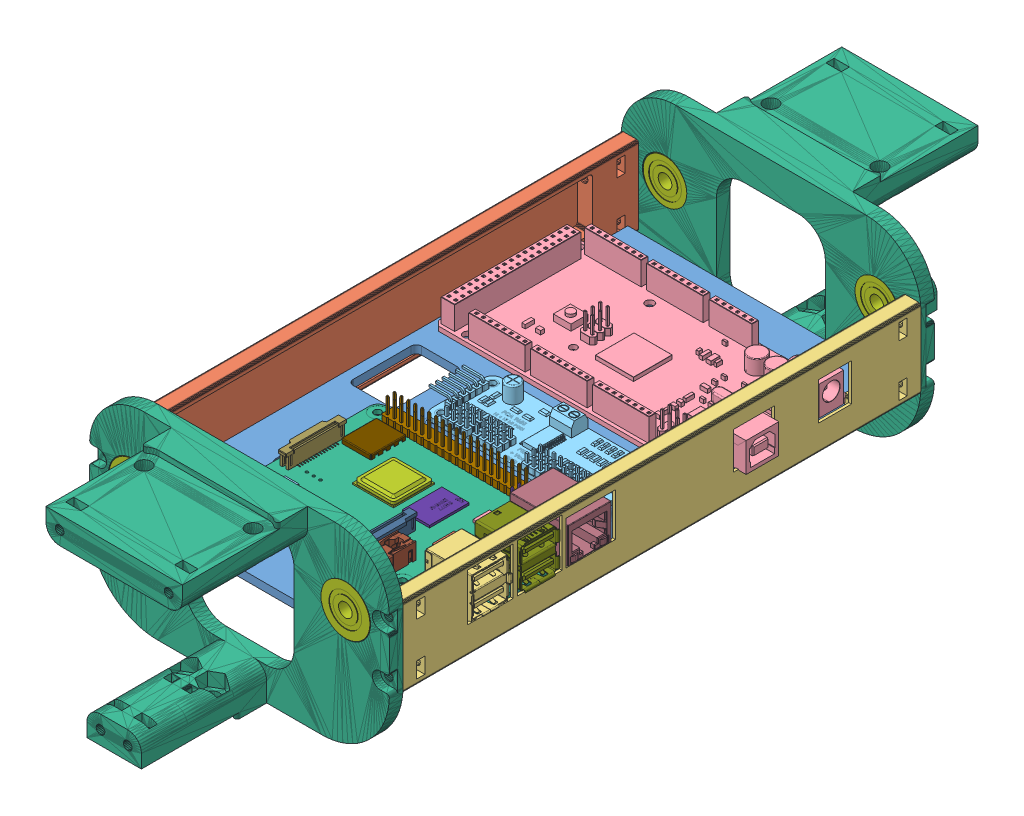
SolidWorks assembly Chase Assembly, configuration Default. Lengths in mm.
Overall size (112.8 70 292).
68 component instances, 28 part files, 131 mates.
Components (placement in the parent):
- 1_2MCU_Plate-1: 1_2MCU_Plate [Default] at (22.3647 94.0168 229.1495) size (106 5.81 180)
- 2_2MCU_Left_side_plate-1: 2_2MCU_Left_side_plate [Default] at (18.1147 57.0168 99.1495) x (1 0 0) z (0 -1 0) size (6.5 190 29)
- 3_2MCU_Right_side_plate-1: 3_2MCU_Right_side_plate [Default] at (121.6147 57.0168 169.1495) x (-1 0 0) z (0 -1 0) size (6.5 190 29)
- ArduinoMega-1: ArduinoMega [Default] at (70.5126 101.4678 88.5891) x (1 0 0) z (0 -1 0) size (107.95 53.42 12.95)
- _Hex_Screws-1: _Hex_Screws [H M3x8] at (55.5647 101.4678 97.3157) x (-0.837169 0 -0.546944) z (-0.546944 0 0.837169) size (5.5 10 6.35) (hidden)
- _Hex_Screws-2: _Hex_Screws [H M3x8] at (55.5647 101.4678 69.2995) x (0.837169 0 0.546944) z (0.546944 0 -0.837169) size (5.5 10 6.35) (hidden)
- 4_M3_nut-1: 4_M3_nut [Default] at (55.5655 95.0168 69.2614) x (0.855198 0 0.518302) z (-0.518302 0 0.855198) size (6 2.34 5.2) (hidden)
- 4_M3_nut-2: 4_M3_nut [Default] at (55.5332 95.0168 97.2415) x (-0.878773 0 0.47724) z (-0.47724 0 -0.878773) size (6 2.34 5.2) (hidden)
- 12Channel PWM-1: 12Channel PWM [Default] at (79.9147 99.8168 132.7995) x (0 0 -1) z (1 0 0) size (25.4 7.55 66.7)
- _M2_nut-1: _M2_nut [Default] at (51.9456 95.5168 142.2881) x (-0.74075 0 -0.671781) z (0 -1 0) size (4.67 4.62 1.63) (hidden)
- _M2_nut-2: _M2_nut [Default] at (107.8452 93.9168 142.288) x (-0.738205 0 -0.674577) z (0 1 0) size (4.67 4.62 1.63) (hidden)
- _M2_nut-3: _M2_nut [Default] at (107.8453 93.9168 123.488) x (-0.739008 0 -0.673697) z (0 1 0) size (4.67 4.62 1.63) (hidden)
- _M2_nut-4: _M2_nut [Default] at (51.8785 93.9168 123.4273) x (-0.741456 0 -0.671001) z (0 1 0) size (4.67 4.62 1.63) (hidden)
- _Hex_Screws-3: _Hex_Screws [H M2x8] at (51.9647 101.3268 142.1995) x (0.837169 0 0.546944) z (0.546944 0 -0.837169) size (4 9.4 4.62) (hidden)
- _Hex_Screws-4: _Hex_Screws [H M2x8] at (107.8647 101.3268 123.3995) x (0.837169 0 0.546944) z (0.546944 0 -0.837169) size (4 9.4 4.62) (hidden)
- _Hex_Screws-5: _Hex_Screws [H M2x8] at (51.9647 101.3268 123.3995) x (0.837169 0 0.546944) z (0.546944 0 -0.837169) size (4 9.4 4.62) (hidden)
- _Hex_Screws-6: _Hex_Screws [H M2x8] at (107.8647 101.3268 142.1995) x (0.837169 0 0.546944) z (0.546944 0 -0.837169) size (4 9.4 4.62) (hidden)
- _Hex_Screws-11: _Hex_Screws [H M2x8] at (40.2647 101.4168 153.7995) x (0.837169 0 0.546944) z (0.546944 0 -0.837169) size (4 9.4 4.62) (hidden)
- _Hex_Screws-12: _Hex_Screws [H M2x8] at (98.2647 101.4068 153.7995) x (0.837169 0 0.546944) z (0.546944 0 -0.837169) size (4 9.4 4.62) (hidden)
- _Hex_Screws-13: _Hex_Screws [H M2x8] at (40.2647 101.4068 202.7995) x (0.837169 0 0.546944) z (0.546944 0 -0.837169) size (4 9.4 4.62) (hidden)
- _Hex_Screws-14: _Hex_Screws [H M2x8] at (98.2647 101.4168 202.7995) x (0.837169 0 0.546944) z (0.546944 0 -0.837169) size (4 9.4 4.62) (hidden)
- _M2_nut-9: _M2_nut [Default] at (98.2838 93.9168 153.7109) x (-0.741324 0 -0.671147) z (0 1 0) size (4.67 4.62 1.63) (hidden)
- _M2_nut-10: _M2_nut [Default] at (40.2838 93.9168 202.711) x (-0.74083 0 -0.671693) z (0 1 0) size (4.67 4.62 1.63) (hidden)
- _M2_nut-11: _M2_nut [Default] at (98.2457 93.9168 202.8881) x (-0.741502 0 -0.670951) z (0 1 0) size (4.67 4.62 1.63) (hidden)
- _M2_nut-12: _M2_nut [Default] at (40.3319 95.5168 153.8603) x (-0.741456 0 -0.671001) z (0 -1 0) size (4.67 4.62 1.63) (hidden)
- Raspberry Pi 4 Model B-1: Raspberry Pi 4 Model B [Default] at (79.2647 100.6168 178.2995) size (89 19.92 58.4)
  - Raspberry Pi 4 Model B.STEP-1: Raspberry Pi 4 Model B.STEP [Default] at origin size (89 19.92 58.4)
    - PCB, RPi4ModelB.STEP-1: PCB, RPi4ModelB.STEP [Default] at origin size (85 1.6 56)
    - Broadcom BCM2711B0 CPU, RPi4ModelB.STEP-1: Broadcom BCM2711B0 CPU, RPi4ModelB.STEP [Default] at (-13.25 0.8 -4.5) size (15 2.3 15)
    - 2.54 mm DUPONT MALE PIN HEADER, POE, 2X2, RPi4ModelB.STEP-1: 2.54 mm DUPONT MALE PIN HEADER, POE, 2X2, RPi4ModelB.STEP [Default] at (19 0.8 -18.36) size (5.08 11.3 5.08)
    - 2.54 mm DUPONT MALE PIN HEADER, IO, 2X20, RPi4ModelB.STEP-1: 2.54 mm DUPONT MALE PIN HEADER, IO, 2X20, RPi4ModelB.STEP [Default] at (-10 0.8 -24.5) size (50.8 11.3 5.08)
    - Camera Connector, RPi4ModelB.STEP-1: Camera Connector, RPi4ModelB.STEP [Default] at (4 0.8 16.5) x (0 0 -1) z (1 0 0) size (22.4 5.68 5.07)
    - Microphone Plug, RPi4ModelB.STEP-1: Microphone Plug, RPi4ModelB.STEP [Default] at (11.5 0.8 21.65) size (7.23 7.55 15)
    - Display Connector, RPi4ModelB.STEP-1: Display Connector, RPi4ModelB.STEP [Default] at (-38.5 0.8 0) x (0 0 1) z (-1 0 0) size (22.4 5.68 5.07)
    - Gigabit Ethernet Port, RPi4ModelB.STEP-1: Gigabit Ethernet Port, RPi4ModelB.STEP [Default] at (45.5 7.55 -17.75) x (0 0 -1) z (1 0 0) size (16.33 17.24 21.6)
    - Female Micro HDMI Connector, RPi4ModelB.STEP-1: Female Micro HDMI Connector, RPi4ModelB.STEP [Default] at (-3 0.8 27.3875) size (6.5 3.51 7.5)
    - Female Micro HDMI Connector, RPi4ModelB.STEP-2: Female Micro HDMI Connector, RPi4ModelB.STEP [Default] at (-16.5 0.8 27.3875) size (6.5 3.51 7.5)
    - Female USB Type C Connector, RPi4ModelB.STEP-1: Female USB Type C Connector, RPi4ModelB.STEP [Default] at (-31.3 0.8 26.5419) size (8.94 3.96 7.9)
    - 2X USB3.0 PORTS, RPi4ModelB.STEP-1: 2X USB3.0 PORTS, RPi4ModelB.STEP [Default] at (37.07 0.8 1) size (17.48 19.42 15.69)
    - 91D77 D9WHV 778K, 4 GB LPDDR4 SDRAM, RPi4ModelB.STEP-1: 91D77 D9WHV 778K, 4 GB LPDDR4 SDRAM, RPi4ModelB.STEP [Default] at (2.25 0.8 -4.5) size (10 0.8 14.5)
    - Cypress CYW43455 Wireless Module Cover, RPi4ModelB.STEP-1: Cypress CYW43455 Wireless Module Cover, RPi4ModelB.STEP [Default] at (-30.5 0.8 -14.5) size (11 1.6 13)
    - SD Card Slot, RPi4ModelB.STEP-1: SD Card Slot, RPi4ModelB.STEP [Default] at (-35.3 -0.8 0) x (0 0 -1) z (-1 0 0) size (11.95 1.45 11.4)
    - VIA VL805 PCIe USB 3.0 controller, RPi4ModelB.STEP-1: VIA VL805 PCIe USB 3.0 controller, RPi4ModelB.STEP [Default] at (17.5 0.8 4) size (8.8 0.8 8.8)
    - 2X USB2.0 PORTS, RPi4ModelB.STEP-1: 2X USB2.0 PORTS, RPi4ModelB.STEP [Default] at (37.065 0.65 19) size (17.87 19.17 15.35)
    - Broadcom BCM54213PE Gigabit Ethernet Transceiver, RPi4ModelB.STEP-1: Broadcom BCM54213PE Gigabit Ethernet Transceiver, RPi4ModelB.STEP [Default] at (16.5 0.8 -10) size (6.8 1 6.8)
    - MxL7704 Universal PMIC, RPi4ModelB.STEP-1: MxL7704 Universal PMIC, RPi4ModelB.STEP [Default] at (-32.5 0.8 16) size (5.4 0.8 5.4)
- 6_Front_shoulder_mg-1: 6_Front_shoulder_mg [Default] at (124.8647 139.0168 39.1495) x (-1 0 0) z (0 -1 0) size (110 51 70)
- 6_Front_shoulder_mg-2: 6_Front_shoulder_mg [Default] at (14.8647 139.0168 229.1495) x (1 0 0) z (0 -1 0) size (110 51 70)
- _Hex_Screws-15: _Hex_Screws [H M3x12] at (18.2198 96.9886 231.1495) x (1 0 0) z (0 1 0) size (5.5 14 6.35) (hidden)
- _Hex_Screws-16: _Hex_Screws [H M3x12] at (121.5159 97.0038 231.1495) x (1 0 0) z (0 1 0) size (5.5 14 6.35) (hidden)
- _Hex_Screws-17: _Hex_Screws [H M3x12] at (18.2375 115.9459 231.1495) x (-0.998805 0.048869 0) z (-0.048869 -0.998805 0) size (5.5 14 6.35) (hidden)
- _Hex_Screws-18: _Hex_Screws [H M3x12] at (18.1956 96.9701 37.1495) x (0.969974 0.243208 0) z (0.243208 -0.969974 0) size (5.5 14 6.35) (hidden)
- _Hex_Screws-19: _Hex_Screws [H M3x12] at (18.1916 115.9399 37.1495) x (1 0 0) z (0 -1 0) size (5.5 14 6.35) (hidden)
- _Hex_Screws-20: _Hex_Screws [H M3x12] at (121.5019 115.9701 231.1495) x (0.105991 0.994367 0) z (-0.994367 0.105991 0) size (5.5 14 6.35) (hidden)
- _Hex_Screws-21: _Hex_Screws [H M3x12] at (121.6489 115.9342 37.1495) x (1 0 0) z (0 -1 0) size (5.5 14 6.35) (hidden)
- _Hex_Screws-22: _Hex_Screws [H M3x12] at (121.6691 96.9226 37.1495) x (1 0 0) z (0 -1 0) size (5.5 14 6.35) (hidden)
- 4_M3_nut-4: 4_M3_nut [Default] at (18.0647 96.9149 222.1495) x (1 0 0) z (0 -1 0) size (6 2.34 5.2) (hidden)
- 4_M3_nut-5: 4_M3_nut [Default] at (18.0647 115.9149 222.1495) x (1 0 0) z (0 -1 0) size (6 2.34 5.2) (hidden)
- 4_M3_nut-6: 4_M3_nut [Default] at (121.6647 96.9149 222.1495) x (1 0 0) z (0 -1 0) size (6 2.34 5.2) (hidden)
- 4_M3_nut-7: 4_M3_nut [Default] at (121.6647 115.9149 222.1495) x (1 0 0) z (0 -1 0) size (6 2.34 5.2) (hidden)
- 4_M3_nut-8: 4_M3_nut [Default] at (18.0647 115.9149 46.1495) x (0.5 0.866025 0) z (-0.866025 0.5 0) size (6 2.34 5.2) (hidden)
- 4_M3_nut-9: 4_M3_nut [Default] at (18.0647 96.9149 44.1495) x (1 0 0) z (0 -1 0) size (6 2.34 5.2) (hidden)
- 4_M3_nut-10: 4_M3_nut [Default] at (121.6647 96.9149 44.1495) x (1 0 0) z (0 -1 0) size (6 2.34 5.2) (hidden)
- 4_M3_nut-11: 4_M3_nut [Default] at (121.6647 115.9149 46.1495) x (0.5 -0.866025 0) z (0.866025 0.5 0) size (6 2.34 5.2) (hidden)
- F625ZZ Ball Bearing-1: F625ZZ Ball Bearing [Default] at (31.004 104.9515 234.1495) x (1 0 0) z (0 0 1) size (18 18 5)
- F625ZZ Ball Bearing-2: F625ZZ Ball Bearing [Default] at (104.9018 120.0403 234.1495) x (-0.879341 -0.476193 0) z (0 0 1) size (18 18 5)
- F625ZZ Ball Bearing-3: F625ZZ Ball Bearing [Default] at (30.2307 104.9537 34.1495) x (-0.995136 0.098516 0) z (0 0 -1) size (18 18 5)
- F625ZZ Ball Bearing-4: F625ZZ Ball Bearing [Default] at (111.8008 105.7118 34.1495) x (-0.923728 -0.383049 0) z (0 0 -1) size (18 18 5)
Mates (geometry in assembly coordinates):
- Coincident1: coincident anti-aligned: plane of 1_2MCU_Plate-1 through (22.3647 94.0168 229.1495) normal (0 -1 0); plane of 2_2MCU_Left_side_plate-1 through (15.8647 94.0168 212.1495) normal (0 1 0)
- Distance8: distance = 1 mm: line of 1_2MCU_Plate-1 through (16.8647 96.9168 56.1495) axis (0 0 1); plane of 2_2MCU_Left_side_plate-1 through (15.8647 100.8703 211.2619) normal (1 0 0)
- Coincident3: coincident anti-aligned: plane of 1_2MCU_Plate-1 through (22.3647 96.9168 56.1495) normal (0 0 -1); plane of 2_2MCU_Left_side_plate-1 through (15.8647 94.0168 56.1495) normal (0 0 1)
- Coincident4: coincident anti-aligned: plane of 1_2MCU_Plate-1 through (22.3647 94.0168 229.1495) normal (0 -1 0); plane of 3_2MCU_Right_side_plate-1 through (123.8647 94.0168 56.1495) normal (0 1 0)
- Distance9: distance = 1 mm anti-aligned: plane of 1_2MCU_Plate-1 through (122.8647 96.9168 229.1495) normal (1 0 0); plane of 3_2MCU_Right_side_plate-1 through (123.8647 100.8703 57.0371) normal (-1 0 0)
- Coincident6: coincident anti-aligned: plane of 1_2MCU_Plate-1 through (22.3647 96.9168 212.1495) normal (0 0 1); plane of 3_2MCU_Right_side_plate-1 through (123.8647 94.0168 212.1495) normal (0 0 -1)
- Coincident8: coincident anti-aligned: plane of 1_2MCU_Plate-1 through (22.3647 99.8168 229.1495) normal (0 1 0); plane of ArduinoMega-1 through (121.3126 99.8168 61.881) normal (0 -1 0)
- Concentric6: concentric aligned: cylinder of 1_2MCU_Plate-1 through (55.5647 94.0168 69.2995) axis (0 1 0) radius 1.6; cylinder of ArduinoMega-1 through (55.5647 99.8158 69.2995) axis (0 1 0) radius 1.5621
- Parallel3: parallel aligned: cylinder of 1_2MCU_Plate-1 through (55.5647 94.0168 97.2995) axis (0 1 0) radius 1.6; cylinder of ArduinoMega-1 through (55.5647 99.8158 97.3157) axis (0 1 0) radius 1.3153
- Concentric8: concentric aligned: circle of ArduinoMega-1; circle of _Hex_Screws-2
- Coincident9: coincident anti-aligned: plane of ArduinoMega-1 through (121.3126 101.4678 61.881) normal (0 1 0); plane of _Hex_Screws-2 through (55.5647 101.4678 69.2995) normal (0 -1 0)
- Concentric9: concentric aligned: circle of ArduinoMega-1; circle of _Hex_Screws-1
- Coincident10: coincident anti-aligned: plane of ArduinoMega-1 through (121.3126 101.4678 61.881) normal (0 1 0); plane of _Hex_Screws-1 through (55.5647 101.4678 97.3157) normal (0 -1 0)
- Distance1: distance = 0.4 mm anti-aligned: plane of 1_2MCU_Plate-1 through (52.489 97.0168 98.9699) normal (0.99966 0 0.026084); plane of 4_M3_nut-2 through (52.9751 97.0168 95.6742) normal (-0.99966 0 -0.026084)
- Coincident15: coincident anti-aligned: plane of 1_2MCU_Plate-1 through (22.3647 97.0168 229.1495) normal (0 -1 0); plane of 4_M3_nut-2 through (55.5332 97.0168 97.2415) normal (0 1 0)
- Distance2: distance = 0.4 mm anti-aligned: plane of 4_M3_nut-2 through (58.1695 97.0168 95.8098) normal (0.522419 0 -0.852689); plane of 1_2MCU_Plate-1 through (55.656 97.0168 93.8007) normal (-0.522419 0 0.852689)
- Distance4: distance = 0.4 mm anti-aligned: plane of 4_M3_nut-1 through (58.1949 97.0168 67.817) normal (0.518302 0 -0.855198); plane of 1_2MCU_Plate-1 through (55.6391 97.0168 65.8003) normal (-0.518302 0 0.855198)
- Distance5: distance = 0.4 mm anti-aligned: plane of 4_M3_nut-1 through (55.6293 97.0168 66.2621) normal (-0.481472 0 -0.876461); plane of 1_2MCU_Plate-1 through (52.5715 97.0168 67.4855) normal (0.481472 0 0.876461)
- Coincident22: coincident anti-aligned: plane of 1_2MCU_Plate-1 through (22.3647 97.0168 229.1495) normal (0 -1 0); plane of 4_M3_nut-1 through (55.5655 97.0168 69.2614) normal (0 1 0)
- Concentric11: concentric aligned: cylinder of 1_2MCU_Plate-1 through (107.8647 94.0168 123.3995) axis (0 1 0) radius 1.2; cylinder of 12Channel PWM-1 through (107.8647 96.2813 123.3995) axis (0 1 0) radius 1.25
- Concentric12: concentric aligned: cylinder of 1_2MCU_Plate-1 through (107.8647 94.0168 142.1995) axis (0 1 0) radius 1.2; cylinder of 12Channel PWM-1 through (107.8647 96.2813 142.1995) axis (0 1 0) radius 1.25
- Coincident24: coincident anti-aligned: plane of 1_2MCU_Plate-1 through (22.3647 99.8168 229.1495) normal (0 1 0); plane of 12Channel PWM-1 through (51.9647 99.8168 123.3995) normal (0 -1 0)
- Concentric13: concentric anti-aligned: cylinder of 12Channel PWM-1 through (51.9647 96.2813 142.1995) axis (0 1 0) radius 1.25; circle of _Hex_Screws-3
- Concentric14: concentric anti-aligned: circle of 12Channel PWM-1; circle of _Hex_Screws-5
- Concentric15: concentric anti-aligned: cylinder of 12Channel PWM-1 through (107.8647 96.2813 123.3995) axis (0 1 0) radius 1.25; circle of _Hex_Screws-4
- Concentric16: concentric anti-aligned: cylinder of 12Channel PWM-1 through (107.8647 96.2813 142.1995) axis (0 1 0) radius 1.25; circle of _Hex_Screws-6
- Coincident26: coincident anti-aligned: plane of 12Channel PWM-1 through (107.8647 101.3268 142.1995) normal (0 1 0); plane of _Hex_Screws-6 through (107.8647 101.3268 142.1995) normal (0 -1 0)
- Coincident27: coincident anti-aligned: plane of 12Channel PWM-1 through (51.9647 101.3268 142.1995) normal (0 1 0); plane of _Hex_Screws-3 through (51.9647 101.3268 142.1995) normal (0 -1 0)
- Coincident28: coincident anti-aligned: plane of 12Channel PWM-1 through (51.9647 101.3268 123.3995) normal (0 1 0); plane of _Hex_Screws-5 through (51.9647 101.3268 123.3995) normal (0 -1 0)
- Coincident29: coincident anti-aligned: plane of 12Channel PWM-1 through (107.8647 101.3268 123.3995) normal (0 1 0); plane of _Hex_Screws-4 through (107.8647 101.3268 123.3995) normal (0 -1 0)
- Tangent4: tangent anti-aligned: plane of 1_2MCU_Plate-1 through (22.3647 95.5168 229.1495) normal (0 -1 0); face of _M2_nut-1
- Tangent5: tangent anti-aligned: plane of 1_2MCU_Plate-1 through (53.7425 95.5168 143.8118) normal (-0.305618 0 -0.952154); edge_curve of _M2_nut-1
- Tangent7: tangent anti-aligned: plane of 1_2MCU_Plate-1 through (22.3647 95.5168 229.1495) normal (0 -1 0); edge_curve of _M2_nut-4
- Tangent8: tangent anti-aligned: plane of 1_2MCU_Plate-1 through (26.8733 95.5168 230.1197) normal (0.977621 0 0.210376); edge_curve of _M2_nut-4
- Tangent9: tangent anti-aligned: plane of 1_2MCU_Plate-1 through (22.3647 95.5168 229.1495) normal (0 -1 0); edge_curve of _M2_nut-3
- Tangent11: tangent anti-aligned: curve of _M2_nut-3; plane of 1_2MCU_Plate-1 through (107.3513 95.5168 125.744) normal (0.673697 0 -0.739008)
- Tangent12: tangent anti-aligned: plane of 1_2MCU_Plate-1 through (109.6383 95.5168 125.0164) normal (-0.303151 0 -0.952943); edge_curve of _M2_nut-3
- Tangent13: tangent anti-aligned: plane of 1_2MCU_Plate-1 through (22.3647 95.5168 229.1495) normal (0 -1 0); edge_curve of _M2_nut-2
- Tangent14: tangent anti-aligned: plane of 1_2MCU_Plate-1 through (107.3485 95.5168 144.5433) normal (0.674577 0 -0.738205); edge_curve of _M2_nut-2
- Tangent15: tangent anti-aligned: plane of 1_2MCU_Plate-1 through (109.6364 95.5168 143.8185) normal (-0.302016 0 -0.953303); edge_curve of _M2_nut-2
- Tangent16: tangent anti-aligned: plane of 1_2MCU_Plate-1 through (51.4573 95.5168 144.5453) normal (0.671781 0 -0.74075); edge_curve of _M2_nut-1
- Tangent17: tangent anti-aligned: plane of 1_2MCU_Plate-1 through (86.9098 95.5168 157.8272) normal (0.671001 0 -0.741456); edge_curve of _M2_nut-4
- Concentric17: concentric aligned: cylinder of 1_2MCU_Plate-1 through (98.2647 94.0168 202.7995) axis (0 1 0) radius 1.3; cylinder of Raspberry Pi 4 Model B-1/Raspberry Pi 4 Model B.STEP-1/PCB, RPi4ModelB.STEP-1 through (98.2647 101.4168 202.7995) axis (0 1 0) radius 1.35
- Coincident30: coincident anti-aligned: plane of 1_2MCU_Plate-1 through (22.3647 99.8168 229.1495) normal (0 1 0); plane of Raspberry Pi 4 Model B-1/Raspberry Pi 4 Model B.STEP-1/PCB, RPi4ModelB.STEP-1 through (79.2647 99.8168 178.2995) normal (0 -1 0)
- Concentric18: concentric aligned: cylinder of 1_2MCU_Plate-1 through (40.2647 94.0168 202.7995) axis (0 1 0) radius 1.3; cylinder of Raspberry Pi 4 Model B-1/Raspberry Pi 4 Model B.STEP-1/PCB, RPi4ModelB.STEP-1 through (40.2647 101.4168 202.7995) axis (0 1 0) radius 1.35
- Tangent18: tangent anti-aligned: plane of 1_2MCU_Plate-1 through (22.3647 95.5168 229.1495) normal (0 -1 0); edge_curve of _M2_nut-11
- Tangent19: tangent anti-aligned: plane of 1_2MCU_Plate-1 through (100.0443 95.5168 204.4098) normal (-0.306684 0 -0.951811); edge_curve of _M2_nut-11
- Tangent20: tangent anti-aligned: plane of 1_2MCU_Plate-1 through (97.76 95.5168 205.1458) normal (0.670951 0 -0.741502); edge_curve of _M2_nut-11
- Tangent21: tangent anti-aligned: plane of 1_2MCU_Plate-1 through (22.3647 95.5168 229.1495) normal (0 -1 0); edge_curve of _M2_nut-10
- Tangent22: tangent anti-aligned: plane of 1_2MCU_Plate-1 through (40.7718 95.5168 200.4537) normal (-0.671693 0 0.74083); edge_curve of _M2_nut-10
- Tangent23: tangent anti-aligned: plane of 1_2MCU_Plate-1 through (38.4867 95.5168 201.1875) normal (0.305731 0 0.952118); edge_curve of _M2_nut-10
- Tangent24: tangent anti-aligned: plane of 1_2MCU_Plate-1 through (22.3647 95.5168 229.1495) normal (0 -1 0); edge_curve of _M2_nut-12
- Tangent25: tangent anti-aligned: plane of 1_2MCU_Plate-1 through (42.0442 95.5168 155.4099) normal (-0.306619 0 -0.951832); edge_curve of _M2_nut-12
- Tangent26: tangent anti-aligned: plane of 1_2MCU_Plate-1 through (42.5491 95.5168 153.0636) normal (-0.977621 0 -0.210376); edge_curve of _M2_nut-12
- Tangent28: tangent anti-aligned: plane of 1_2MCU_Plate-1 through (22.3647 95.5168 229.1495) normal (0 -1 0); edge_curve of _M2_nut-9
- Tangent29: tangent anti-aligned: plane of 1_2MCU_Plate-1 through (98.7701 95.5168 151.4533) normal (-0.671147 0 0.741324); edge_curve of _M2_nut-9
- Tangent30: tangent anti-aligned: plane of 1_2MCU_Plate-1 through (96.4855 95.5168 152.1888) normal (0.306432 0 0.951893); edge_curve of _M2_nut-9
- Concentric19: concentric anti-aligned: cylinder of 1_2MCU_Plate-1 through (40.2647 94.0168 202.7995) axis (0 1 0) radius 1.3; circle of _Hex_Screws-13
- Concentric20: concentric anti-aligned: cylinder of 1_2MCU_Plate-1 through (40.2647 94.0168 153.7995) axis (0 1 0) radius 1.3; circle of _Hex_Screws-11
- Concentric21: concentric anti-aligned: cylinder of 1_2MCU_Plate-1 through (98.2647 94.0168 202.7995) axis (0 1 0) radius 1.3; circle of _Hex_Screws-14
- Concentric22: concentric anti-aligned: cylinder of 1_2MCU_Plate-1 through (98.2647 94.0168 153.7995) axis (0 1 0) radius 1.3; circle of _Hex_Screws-12
- Coincident31: coincident anti-aligned: plane of _Hex_Screws-14 through (98.2647 101.4168 202.7995) normal (0 -1 0); plane of Raspberry Pi 4 Model B-1/Raspberry Pi 4 Model B.STEP-1/PCB, RPi4ModelB.STEP-1 through (79.2647 101.4168 178.2995) normal (0 1 0)
- Coincident32: coincident anti-aligned: plane of _Hex_Screws-13 through (40.2647 101.4068 202.7995) normal (0 -1 0); plane of Raspberry Pi 4 Model B-1/Raspberry Pi 4 Model B.STEP-1/PCB, RPi4ModelB.STEP-1 through (40.2647 101.4068 202.7995) normal (0 1 0)
- Coincident33: coincident anti-aligned: plane of _Hex_Screws-11 through (40.2647 101.4168 153.7995) normal (0 -1 0); plane of Raspberry Pi 4 Model B-1/Raspberry Pi 4 Model B.STEP-1/PCB, RPi4ModelB.STEP-1 through (79.2647 101.4168 178.2995) normal (0 1 0)
- Coincident34: coincident anti-aligned: plane of _Hex_Screws-12 through (98.2647 101.4068 153.7995) normal (0 -1 0); plane of Raspberry Pi 4 Model B-1/Raspberry Pi 4 Model B.STEP-1/PCB, RPi4ModelB.STEP-1 through (98.2647 101.4068 153.7995) normal (0 1 0)
- Coincident35: coincident anti-aligned: plane of 2_2MCU_Left_side_plate-1 through (18.1147 57.0168 229.1495) normal (0 0 1); plane of 6_Front_shoulder_mg-2 through (14.8647 139.0168 229.1495) normal (0 0 -1)
- Distance6: distance = 0 mm aligned: plane of 3_2MCU_Right_side_plate-1 through (124.8647 120.0168 229.1495) normal (1 0 0); plane of 6_Front_shoulder_mg-2 through (124.8647 139.0168 229.1495) normal (1 0 0)
- Distance7: distance = 18 mm aligned: plane of 6_Front_shoulder_mg-2 through (14.8647 139.0168 229.1495) normal (0 1 0); plane of 3_2MCU_Right_side_plate-1 through (119.3647 121.0168 229.1495) normal (0 1 0)
- Coincident39: coincident anti-aligned: plane of 3_2MCU_Right_side_plate-1 through (121.6147 57.0168 39.1495) normal (0 0 -1); plane of 6_Front_shoulder_mg-1 through (124.8647 139.0168 39.1495) normal (0 0 1)
- Distance10: distance = 18 mm aligned: plane of 6_Front_shoulder_mg-1 through (124.8647 139.0168 39.1495) normal (0 1 0); plane of 2_2MCU_Left_side_plate-1 through (20.3647 121.0168 39.1495) normal (0 1 0)
- Coincident41: coincident aligned: plane of 2_2MCU_Left_side_plate-1 through (14.8647 120.0168 39.1495) normal (-1 0 0); plane of 6_Front_shoulder_mg-1 through (14.8647 139.0168 39.1495) normal (-1 0 0)
- Distance11: distance = 0.2 mm anti-aligned: plane of 3_2MCU_Right_side_plate-1 through (124.8647 113.1168 221.1495) normal (0 1 0); plane of 4_M3_nut-7 through (120.1647 113.3168 224.1495) normal (0 -1 0)
- Distance12: distance = 0.2 mm: plane of 3_2MCU_Right_side_plate-1 through (124.8647 120.0168 229.1495) normal (1 0 0); line of 4_M3_nut-7 through (124.6647 115.9149 223.9175) axis (0 0 -1)
- Coincident45: coincident anti-aligned: plane of 3_2MCU_Right_side_plate-1 through (124.8647 113.1168 224.1495) normal (0 0 -1); plane of 4_M3_nut-7 through (121.6647 115.9149 224.1495) normal (0 0 1)
- Distance13: distance = 0.2 mm anti-aligned: plane of 4_M3_nut-6 through (120.1647 94.3168 224.1495) normal (0 -1 0); plane of 3_2MCU_Right_side_plate-1 through (124.8647 94.1168 221.1495) normal (0 1 0)
- Distance14: distance = 0.2 mm: line of 4_M3_nut-6 through (124.6647 96.9149 223.9175) axis (0 0 -1); plane of 3_2MCU_Right_side_plate-1 through (124.8647 120.0168 229.1495) normal (1 0 0)
- Coincident48: coincident anti-aligned: plane of 3_2MCU_Right_side_plate-1 through (124.8647 94.1168 224.1495) normal (0 0 -1); plane of 4_M3_nut-6 through (121.6647 96.9149 224.1495) normal (0 0 1)
- Distance15: distance = 0.2 mm anti-aligned: plane of 4_M3_nut-5 through (16.5647 113.3168 224.1495) normal (0 -1 0); plane of 2_2MCU_Left_side_plate-1 through (14.8647 113.1168 224.1495) normal (0 1 0)
- Distance16: distance = 0.2 mm: line of 4_M3_nut-5 through (15.0647 115.9149 223.9175) axis (0 0 -1); plane of 2_2MCU_Left_side_plate-1 through (14.8647 120.0168 39.1495) normal (-1 0 0)
- Coincident51: coincident anti-aligned: plane of 2_2MCU_Left_side_plate-1 through (14.8647 118.9168 224.1495) normal (0 0 -1); plane of 4_M3_nut-5 through (18.0647 115.9149 224.1495) normal (0 0 1)
- Distance17: distance = 0.2 mm anti-aligned: plane of 4_M3_nut-4 through (16.5647 94.3168 224.1495) normal (0 -1 0); plane of 2_2MCU_Left_side_plate-1 through (14.8647 94.1168 224.1495) normal (0 1 0)
- Distance18: distance = 0.2 mm: plane of 2_2MCU_Left_side_plate-1 through (14.8647 120.0168 39.1495) normal (-1 0 0); line of 4_M3_nut-4 through (15.0647 96.9149 223.9175) axis (0 0 -1)
- Coincident54: coincident anti-aligned: plane of 2_2MCU_Left_side_plate-1 through (14.8647 99.9168 224.1495) normal (0 0 -1); plane of 4_M3_nut-4 through (18.0647 96.9149 224.1495) normal (0 0 1)
- Distance19: distance = 0.2 mm anti-aligned: plane of 4_M3_nut-11 through (123.1647 113.3168 44.1495) normal (0 -1 0); plane of 3_2MCU_Right_side_plate-1 through (124.8647 113.1168 44.1495) normal (0 1 0)
- Distance20: distance = 0.2 mm: line of 4_M3_nut-11 through (124.6647 115.9149 44.3816) axis (0 0 1); plane of 3_2MCU_Right_side_plate-1 through (124.8647 120.0168 229.1495) normal (1 0 0)
- Coincident57: coincident anti-aligned: plane of 3_2MCU_Right_side_plate-1 through (124.8647 118.9168 44.1495) normal (0 0 1); plane of 4_M3_nut-11 through (121.6647 115.9149 44.1495) normal (0 0 -1)
- Distance21: distance = 0.2 mm anti-aligned: plane of 4_M3_nut-10 through (120.1647 94.3168 46.1495) normal (0 -1 0); plane of 3_2MCU_Right_side_plate-1 through (124.8647 94.1168 44.1495) normal (0 1 0)
- Distance22: distance = 0.2 mm: line of 4_M3_nut-10 through (124.6647 96.9149 45.9175) axis (0 0 -1); plane of 3_2MCU_Right_side_plate-1 through (124.8647 120.0168 229.1495) normal (1 0 0)
- Coincident60: coincident anti-aligned: plane of 3_2MCU_Right_side_plate-1 through (124.8647 99.9168 44.1495) normal (0 0 1); plane of 4_M3_nut-10 through (121.6647 96.9149 44.1495) normal (0 0 -1)
- Distance23: distance = 0.2 mm anti-aligned: plane of 4_M3_nut-8 through (19.5647 113.3168 44.1495) normal (0 -1 0); plane of 2_2MCU_Left_side_plate-1 through (14.8647 113.1168 47.1495) normal (0 1 0)
- Distance24: distance = 0.2 mm: line of 4_M3_nut-8 through (15.0647 115.9149 44.3816) axis (0 0 1); plane of 2_2MCU_Left_side_plate-1 through (14.8647 120.0168 39.1495) normal (-1 0 0)
- Coincident63: coincident anti-aligned: plane of 2_2MCU_Left_side_plate-1 through (14.8647 113.1168 44.1495) normal (0 0 1); plane of 4_M3_nut-8 through (18.0647 115.9149 44.1495) normal (0 0 -1)
- Distance25: distance = 0.2 mm anti-aligned: plane of 4_M3_nut-9 through (16.5647 94.3168 46.1495) normal (0 -1 0); plane of 2_2MCU_Left_side_plate-1 through (14.8647 94.1168 47.1495) normal (0 1 0)
- Distance26: distance = 0.2 mm: line of 4_M3_nut-9 through (15.0647 96.9149 45.9175) axis (0 0 -1); plane of 2_2MCU_Left_side_plate-1 through (14.8647 120.0168 39.1495) normal (-1 0 0)
- Coincident66: coincident anti-aligned: plane of 2_2MCU_Left_side_plate-1 through (14.8647 94.1168 44.1495) normal (0 0 1); plane of 4_M3_nut-9 through (18.0647 96.9149 44.1495) normal (0 0 -1)
- Coincident70: coincident anti-aligned: plane of 6_Front_shoulder_mg-2 through (14.8647 139.0168 231.1495) normal (0 0 1); plane of _Hex_Screws-17 through (18.2375 115.9459 231.1495) normal (0 0 -1)
- Tangent35: tangent anti-aligned: plane of 6_Front_shoulder_mg-2 through (18.1036 114.4153 229.1495) normal (-0.130528 0.991445 0); cylinder of _Hex_Screws-17 through (18.2375 115.9459 219.1495) axis (0 0 1) radius 1.5
- Tangent36: tangent anti-aligned: plane of 6_Front_shoulder_mg-2 through (10.9726 137.4046 229.1495) normal (-0.923879 -0.382685 0); cylinder of _Hex_Screws-17 through (18.2375 115.9459 219.1495) axis (0 0 1) radius 1.5
- Coincident72: coincident anti-aligned: plane of 6_Front_shoulder_mg-2 through (14.8647 139.0168 231.1495) normal (0 0 1); plane of _Hex_Screws-15 through (18.2198 96.9886 231.1495) normal (0 0 -1)
- Tangent37: tangent anti-aligned: plane of 6_Front_shoulder_mg-2 through (37.3192 109.7534 229.1495) normal (-0.608761 0.793354 0); cylinder of _Hex_Screws-15 through (18.2198 96.9886 219.1495) axis (0 0 1) radius 1.5
- Tangent38: tangent anti-aligned: plane of 6_Front_shoulder_mg-2 through (4.255 134.6221 229.1495) normal (-0.923879 -0.382685 0); cylinder of _Hex_Screws-15 through (18.2198 96.9886 219.1495) axis (0 0 1) radius 1.5
- Tangent39: tangent anti-aligned: plane of 6_Front_shoulder_mg-2 through (21.7588 155.6609 229.1495) normal (0.382679 0.923881 0); cylinder of _Hex_Screws-20 through (121.5019 115.9701 219.1495) axis (0 0 1) radius 1.5
- Coincident73: coincident anti-aligned: plane of 6_Front_shoulder_mg-2 through (14.8647 139.0168 231.1495) normal (0 0 1); plane of _Hex_Screws-20 through (121.5019 115.9701 231.1495) normal (0 0 -1)
- Tangent40: tangent anti-aligned: plane of 6_Front_shoulder_mg-2 through (112.648 98.5143 229.1495) normal (0.923882 -0.382678 0); cylinder of _Hex_Screws-20 through (121.5019 115.9701 219.1495) axis (0 0 1) radius 1.5
- Coincident74: coincident anti-aligned: plane of 6_Front_shoulder_mg-2 through (14.8647 139.0168 231.1495) normal (0 0 1); plane of _Hex_Screws-16 through (121.5159 97.0038 231.1495) normal (0 0 -1)
- Tangent41: tangent anti-aligned: plane of 6_Front_shoulder_mg-2 through (60.5122 174.0427 229.1495) normal (0.793359 0.608754 0); cylinder of _Hex_Screws-16 through (121.5159 97.0038 219.1495) axis (0 0 1) radius 1.5
- Tangent42: tangent anti-aligned: plane of 6_Front_shoulder_mg-2 through (119.3655 95.7319 229.1495) normal (0.923882 -0.382678 0); cylinder of _Hex_Screws-16 through (121.5159 97.0038 219.1495) axis (0 0 1) radius 1.5
- Coincident75: coincident anti-aligned: plane of 6_Front_shoulder_mg-1 through (124.8647 139.0168 37.1495) normal (0 0 -1); plane of _Hex_Screws-19 through (18.1916 115.9399 37.1495) normal (0 0 1)
- Tangent43: tangent anti-aligned: plane of 6_Front_shoulder_mg-1 through (126.2295 128.6509 39.1495) normal (-0.130531 0.991444 0); cylinder of _Hex_Screws-19 through (18.1916 115.9399 49.1495) axis (0 0 -1) radius 1.5
- Tangent44: tangent anti-aligned: plane of 6_Front_shoulder_mg-1 through (24.4831 152.2334 39.1495) normal (-0.991443 0.130537 0); cylinder of _Hex_Screws-19 through (18.1916 115.9399 49.1495) axis (0 0 -1) radius 1.5
- Coincident76: coincident anti-aligned: plane of 6_Front_shoulder_mg-1 through (124.8647 139.0168 37.1495) normal (0 0 -1); plane of _Hex_Screws-18 through (18.1956 96.9701 37.1495) normal (0 0 1)
- Tangent45: tangent anti-aligned: plane of 6_Front_shoulder_mg-1 through (106.5545 162.8792 39.1495) normal (-0.60876 0.793355 0); cylinder of _Hex_Screws-18 through (18.1956 96.9701 49.1495) axis (0 0 -1) radius 1.5
- Tangent46: tangent anti-aligned: plane of 6_Front_shoulder_mg-1 through (26.942 151.9095 39.1495) normal (-0.991444 0.130536 0); cylinder of _Hex_Screws-18 through (18.1956 96.9701 49.1495) axis (0 0 -1) radius 1.5
- Coincident77: coincident anti-aligned: plane of 6_Front_shoulder_mg-1 through (124.8647 139.0168 37.1495) normal (0 0 -1); plane of _Hex_Screws-21 through (121.6489 115.9342 37.1495) normal (0 0 1)
- Tangent47: tangent anti-aligned: plane of 6_Front_shoulder_mg-1 through (127.9929 115.2565 39.1495) normal (-0.130528 0.991445 0); cylinder of _Hex_Screws-21 through (121.6489 115.9342 49.1495) axis (0 0 -1) radius 1.5
- Tangent48: tangent anti-aligned: plane of 6_Front_shoulder_mg-1 through (135.7341 124.8515 39.1495) normal (-0.608761 0.793353 0); cylinder of _Hex_Screws-21 through (121.6489 115.9342 49.1495) axis (0 0 -1) radius 1.5
- Coincident78: coincident anti-aligned: plane of 6_Front_shoulder_mg-1 through (124.8647 139.0168 37.1495) normal (0 0 -1); plane of _Hex_Screws-22 through (121.6691 96.9226 37.1495) normal (0 0 1)
- Tangent49: tangent anti-aligned: plane of 6_Front_shoulder_mg-1 through (119.1674 95.739 39.1495) normal (0.13052 0.991446 0); cylinder of _Hex_Screws-22 through (121.6691 96.9226 49.1495) axis (0 0 -1) radius 1.5
- Tangent50: tangent anti-aligned: plane of 6_Front_shoulder_mg-1 through (138.4056 133.4079 39.1495) normal (-0.923878 0.382688 0); cylinder of _Hex_Screws-22 through (121.6691 96.9226 49.1495) axis (0 0 -1) radius 1.5
- Tangent51: tangent anti-aligned: plane of 6_Front_shoulder_mg-2 through (54.7421 169.8089 229.1495) normal (0.791499 0.611171 0); cylinder of F625ZZ Ball Bearing-2 through (108.7113 113.0056 231.1495) axis (0 0 -1) radius 8
- Coincident79: coincident anti-aligned: plane of 6_Front_shoulder_mg-2 through (14.8647 139.0168 233.1495) normal (0 0 1); plane of F625ZZ Ball Bearing-2 through (112.5209 105.9708 233.1495) normal (0 0 -1)
- Tangent52: tangent anti-aligned: plane of 6_Front_shoulder_mg-2 through (90.3572 96.6481 229.1495) normal (0.872048 -0.48942 0); cylinder of F625ZZ Ball Bearing-2 through (108.7113 113.0056 231.1495) axis (0 0 -1) radius 8
- Coincident80: coincident anti-aligned: plane of 6_Front_shoulder_mg-2 through (14.8647 139.0168 233.1495) normal (0 0 1); plane of F625ZZ Ball Bearing-1 through (31.004 120.9515 233.1495) normal (0 0 -1)
- Tangent53: tangent anti-aligned: plane of 6_Front_shoulder_mg-2 through (35.0025 106.0196 229.1495) normal (-0.520939 0.853594 0); cylinder of F625ZZ Ball Bearing-1 through (31.004 112.9515 231.1495) axis (0 0 -1) radius 8
- Tangent54: tangent anti-aligned: plane of 6_Front_shoulder_mg-2 through (34.8219 141.9539 229.1495) normal (-0.989343 -0.1456 0); cylinder of F625ZZ Ball Bearing-1 through (31.004 112.9515 231.1495) axis (0 0 -1) radius 8
- Coincident81: coincident anti-aligned: plane of 6_Front_shoulder_mg-1 through (124.8647 139.0168 35.1495) normal (0 0 -1); plane of F625ZZ Ball Bearing-4 through (105.6721 120.4915 35.1495) normal (0 0 1)
- Tangent55: tangent anti-aligned: plane of 6_Front_shoulder_mg-1 through (100.7364 139.0168 39.1495) normal (1 0 0); cylinder of F625ZZ Ball Bearing-4 through (108.7364 113.1016 37.1495) axis (0 0 1) radius 8
- Tangent56: tangent anti-aligned: plane of 6_Front_shoulder_mg-1 through (128.597 130.2338 39.1495) normal (0.391104 -0.920346 0); cylinder of F625ZZ Ball Bearing-4 through (108.7364 113.1016 37.1495) axis (0 0 1) radius 8
- Coincident82: coincident anti-aligned: plane of 6_Front_shoulder_mg-1 through (124.8647 139.0168 35.1495) normal (0 0 -1); plane of F625ZZ Ball Bearing-3 through (31.8069 120.8759 35.1495) normal (0 0 1)
- Tangent57: tangent anti-aligned: cylinder of F625ZZ Ball Bearing-3 through (31.0188 112.9148 37.1495) axis (0 0 1) radius 8; plane of 6_Front_shoulder_mg-1 through (127.8839 122.6716 39.1495) normal (-0.181639 0.983365 0)
- Tangent58: tangent anti-aligned: plane of 6_Front_shoulder_mg-1 through (37.7245 119.6053 39.1495) normal (-0.976075 -0.217433 0); cylinder of F625ZZ Ball Bearing-3 through (31.0188 112.9148 37.1495) axis (0 0 1) radius 8
